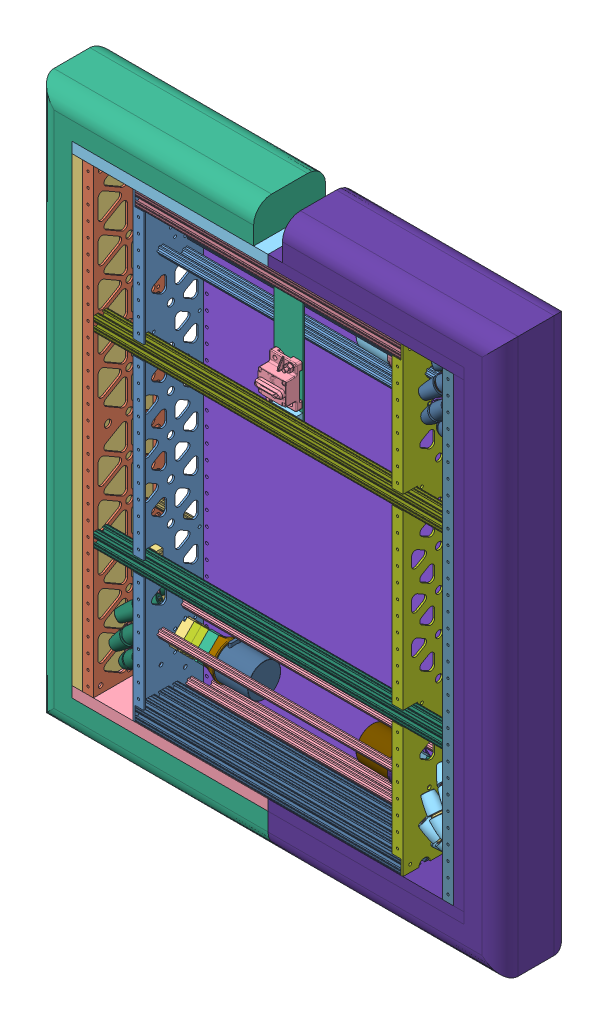
SolidWorks assembly Copy of Fame 2020, configuration Default. Lengths in mm.
Overall size (819.15 977.9 171.99).
407 component instances, 94 part files, 0 mates.
Components (placement in the parent):
- Inner plate v12(Mirror)^Copy of Fame 2020-1: Inner plate v12(Mirror)^Copy of Fame 2020 [Default] at (-212.725 0 58.7875) x (0 1 0) z (0 0 -1) size (812.8 19.05 127) (virtual)
  - Inner plate v12(Mirror)-0^Inner plate v12(Mirror)_Copy of Fame 2020-1: Inner plate v12(Mirror)-0^Inner plate v12(Mirror)_Copy of Fame 2020 [Default] at origin size (812.8 19.05 127) (virtual)
- Outer plate v11(Mirror)^Copy of Fame 2020-1: Outer plate v11(Mirror)^Copy of Fame 2020 [Default] at (-333.375 0 58.7875) x (0 -1 0) z (0 0 -1) size (812.8 19.05 127) (virtual)
  - Outer plate v11(Mirror)-1^Outer plate v11(Mirror)_Copy of Fame 2020-1: Outer plate v11(Mirror)-1^Outer plate v11(Mirror)_Copy of Fame 2020 [Default] at origin size (812.8 19.05 127) (virtual)
- Bumper Assembly v4(Mirror)^Copy of Fame 2020-1: Bumper Assembly v4(Mirror)^Copy of Fame 2020 [Default] at (-327.025 0.0665 58.7875) x (-1 0 0) z (0 0 -1) size (409.58 977.9 127) (virtual)
  - Bumper Assembly v4(Mirror)-2^Bumper Assembly v4(Mirror)_Copy of Fame 2020-1: Bumper Assembly v4(Mirror)-2^Bumper Assembly v4(Mirror)_Copy of Fame 2020 [Default] at origin size (19.05 812.8 127) (virtual)
  - Bumper Assembly v4(Mirror)-3^Bumper Assembly v4(Mirror)_Copy of Fame 2020-1: Bumper Assembly v4(Mirror)-3^Bumper Assembly v4(Mirror)_Copy of Fame 2020 [Default] at origin size (346.08 19.05 127) (virtual)
  - Bumper Assembly v4(Mirror)-4^Bumper Assembly v4(Mirror)_Copy of Fame 2020-1: Bumper Assembly v4(Mirror)-4^Bumper Assembly v4(Mirror)_Copy of Fame 2020 [Default] at origin size (346.08 19.05 127) (virtual)
  - Bumper Assembly v4(Mirror)-5^Bumper Assembly v4(Mirror)_Copy of Fame 2020-1: Bumper Assembly v4(Mirror)-5^Bumper Assembly v4(Mirror)_Copy of Fame 2020 [Default] at origin size (409.58 977.9 127) (virtual)
- NEO Gearbox 2-stage Custom^Copy of Fame 2020-1: NEO Gearbox 2-stage Custom^Copy of Fame 2020 [Default] at (0 0 425) size (164.9 90.53 90.53) (virtual)
  - VersaPlanetary_4_1_Gear_Kit_217-2818^NEO Gearbox 2-stage Custom_Copy of Fame 2020-1: VersaPlanetary_4_1_Gear_Kit_217-2818^NEO Gearbox 2-stage Custom_Copy of Fame 2020 [Default] at (-15.25 22.225 0) x (0 -0.707107 0.707107) z (-1 0 0) size (35.49 35.49 17.4) (virtual)
    - 217-2725-001 Rev1_24t Sun^VersaPlanetary_4_1_Gear_Kit_217-2818_NEO Gearbox 2-stage Custom_Copy of Fame 2020-1: 217-2725-001 Rev1_24t Sun^VersaPlanetary_4_1_Gear_Kit_217-2818_NEO Gearbox 2-stage Custom_Copy of Fame 2020 [Default] at (-36.69 -517.1337 -209.675) x (0.707107 0.707107 0) z (0 0 1) size (14.4 14.45 12.7) (virtual)
    - 217-2725-002 Rev1_24t Planet^VersaPlanetary_4_1_Gear_Kit_217-2818_NEO Gearbox 2-stage Custom_Copy of Fame 2020-1: 217-2725-002 Rev1_24t Planet^VersaPlanetary_4_1_Gear_Kit_217-2818_NEO Gearbox 2-stage Custom_Copy of Fame 2020 [Default] at (-45.2382 -525.6819 -212.025) x (-0.793353 0.608761 0) z (0 0 -1) size (13.12 13.1 8) (virtual)
    - 217-2724-002 Rev1^VersaPlanetary_4_1_Gear_Kit_217-2818_NEO Gearbox 2-stage Custom_Copy of Fame 2020-1: 217-2724-002 Rev1^VersaPlanetary_4_1_Gear_Kit_217-2818_NEO Gearbox 2-stage Custom_Copy of Fame 2020 [Default] at (-36.69 -517.1337 -218.375) x (1 0 0) z (0 0 -1) size (34.7 34.7 4.7) (virtual)
    - 217-2625-010 Rev1^VersaPlanetary_4_1_Gear_Kit_217-2818_NEO Gearbox 2-stage Custom_Copy of Fame 2020-1: 217-2625-010 Rev1^VersaPlanetary_4_1_Gear_Kit_217-2818_NEO Gearbox 2-stage Custom_Copy of Fame 2020 [Default] at (-45.2382 -525.6819 -214.725) x (0.854322 0.519745 0) z (0 0 1) size (4 4 12) (virtual)
    - 217-2725-002 Rev1_24t Planet^VersaPlanetary_4_1_Gear_Kit_217-2818_NEO Gearbox 2-stage Custom_Copy of Fame 2020-2: 217-2725-002 Rev1_24t Planet^VersaPlanetary_4_1_Gear_Kit_217-2818_NEO Gearbox 2-stage Custom_Copy of Fame 2020 [Default] at (-28.1418 -525.6819 -212.025) x (-0.608761 -0.793353 0) z (0 0 -1) size (13.12 13.1 8) (virtual)
    - 217-2725-002 Rev1_24t Planet^VersaPlanetary_4_1_Gear_Kit_217-2818_NEO Gearbox 2-stage Custom_Copy of Fame 2020-3: 217-2725-002 Rev1_24t Planet^VersaPlanetary_4_1_Gear_Kit_217-2818_NEO Gearbox 2-stage Custom_Copy of Fame 2020 [Default] at (-28.1418 -508.5855 -212.025) x (0.793353 -0.608761 0) z (0 0 -1) size (13.12 13.1 8) (virtual)
    - 217-2725-002 Rev1_24t Planet^VersaPlanetary_4_1_Gear_Kit_217-2818_NEO Gearbox 2-stage Custom_Copy of Fame 2020-4: 217-2725-002 Rev1_24t Planet^VersaPlanetary_4_1_Gear_Kit_217-2818_NEO Gearbox 2-stage Custom_Copy of Fame 2020 [Default] at (-45.2382 -508.5855 -212.025) x (0.608761 0.793353 0) z (0 0 -1) size (13.12 13.1 8) (virtual)
    - 217-2625-010 Rev1^VersaPlanetary_4_1_Gear_Kit_217-2818_NEO Gearbox 2-stage Custom_Copy of Fame 2020-2: 217-2625-010 Rev1^VersaPlanetary_4_1_Gear_Kit_217-2818_NEO Gearbox 2-stage Custom_Copy of Fame 2020 [Default] at (-28.1418 -525.6819 -214.725) x (-0.519745 0.854322 0) z (0 0 1) size (4 4 12) (virtual)
    - 217-2625-010 Rev1^VersaPlanetary_4_1_Gear_Kit_217-2818_NEO Gearbox 2-stage Custom_Copy of Fame 2020-3: 217-2625-010 Rev1^VersaPlanetary_4_1_Gear_Kit_217-2818_NEO Gearbox 2-stage Custom_Copy of Fame 2020 [Default] at (-28.1418 -508.5855 -214.725) x (-0.854322 -0.519745 0) z (0 0 1) size (4 4 12) (virtual)
    - 217-2625-010 Rev1^VersaPlanetary_4_1_Gear_Kit_217-2818_NEO Gearbox 2-stage Custom_Copy of Fame 2020-4: 217-2625-010 Rev1^VersaPlanetary_4_1_Gear_Kit_217-2818_NEO Gearbox 2-stage Custom_Copy of Fame 2020 [Default] at (-45.2382 -508.5855 -214.725) x (0.519745 -0.854322 0) z (0 0 1) size (4 4 12) (virtual)
  - 217-2625-026 Rev1^NEO Gearbox 2-stage Custom_Copy of Fame 2020-1: 217-2625-026 Rev1^NEO Gearbox 2-stage Custom_Copy of Fame 2020 [Default] at (211.875 -317.5 -391.6125) x (0 -0.707107 0.707107) z (-1 0 0) size (44.45 42 18.12) (virtual)
  - 217-2742-001 Rev4^NEO Gearbox 2-stage Custom_Copy of Fame 2020-1: 217-2742-001 Rev4^NEO Gearbox 2-stage Custom_Copy of Fame 2020 [Default] at (218.5752 -317.5 -391.6125) x (1 0 0) z (0 0.63857 0.769564) size (7 28 28) (virtual)
  - 217-2742-001 Rev4^NEO Gearbox 2-stage Custom_Copy of Fame 2020-2: 217-2742-001 Rev4^NEO Gearbox 2-stage Custom_Copy of Fame 2020 [Default] at (226.5752 -317.5 -391.6125) x (1 0 0) z (0 0.707107 0.707107) size (7 28 28) (virtual)
  - 217-2625-017 Rev1_9714K61^NEO Gearbox 2-stage Custom_Copy of Fame 2020-1: 217-2625-017 Rev1_9714K61^NEO Gearbox 2-stage Custom_Copy of Fame 2020 [Default] at (225.795 -317.6887 -391.9075) x (0 0.983393 0.181491) z (0 -0.181491 0.983393) size (28.51 4.98 27.43) (virtual)
  - 217-2625-025 Rev1^NEO Gearbox 2-stage Custom_Copy of Fame 2020-1: 217-2625-025 Rev1^NEO Gearbox 2-stage Custom_Copy of Fame 2020 [Default] at (182.475 -317.5 -391.6125) x (0 -0.707107 0.707107) z (-1 0 0) size (44.45 42 18) (virtual)
  - 217-2816-001 Rev1^NEO Gearbox 2-stage Custom_Copy of Fame 2020-1: 217-2816-001 Rev1^NEO Gearbox 2-stage Custom_Copy of Fame 2020 [Default] at (212.025 -317.5 -391.6125) x (0 -0.707107 0.707107) z (1 0 0) size (42 42 14.5) (virtual)
  - 217-2816-001 Rev1^NEO Gearbox 2-stage Custom_Copy of Fame 2020-2: 217-2816-001 Rev1^NEO Gearbox 2-stage Custom_Copy of Fame 2020 [Default] at (199.325 -317.5 -391.6125) x (0 -0.707107 0.707107) z (1 0 0) size (42 42 14.5) (virtual)
  - 217-4649-001 Rev1^NEO Gearbox 2-stage Custom_Copy of Fame 2020-1: 217-4649-001 Rev1^NEO Gearbox 2-stage Custom_Copy of Fame 2020 [Default] at (185.629 -317.5 -391.6125) x (0 -0.707107 0.707107) z (1 0 0) size (18 18 13) (virtual)
  - VersaPlanetary_CIM_Adapter_217-4018^NEO Gearbox 2-stage Custom_Copy of Fame 2020-1: VersaPlanetary_CIM_Adapter_217-4018^NEO Gearbox 2-stage Custom_Copy of Fame 2020 [Default] at (165.15 -317.5 -391.6125) x (0 -0.707107 0.707107) z (0 0.707107 0.707107) size (64.01 21.55 64.01) (virtual)
  - NEO Motor REV-21-1650^NEO Gearbox 2-stage Custom_Copy of Fame 2020-1: NEO Motor REV-21-1650^NEO Gearbox 2-stage Custom_Copy of Fame 2020 [Default] at (153.625 -317.5 -391.6125) x (0 -0.707107 -0.707107) z (1 0 0) size (61.14 61.02 93.25) (virtual)
  - 3_1 Output Shaft Custom^NEO Gearbox 2-stage Custom_Copy of Fame 2020-1: 3_1 Output Shaft Custom^NEO Gearbox 2-stage Custom_Copy of Fame 2020 [Default] at (211.3752 -317.5 -391.6125) x (1 0 0) z (0 0.707107 0.707107) size (48.9 34.7 34.7) (virtual)
- Left Wheel Assembly^Copy of Fame 2020-1: Left Wheel Assembly^Copy of Fame 2020 [Default] at (500 0 0) size (65.82 166.11 165.01) (virtual)
  - 6_Mecanum_Wheel_Left_217-2799^Left Wheel Assembly_Copy of Fame 2020-1: 6_Mecanum_Wheel_Left_217-2799^Left Wheel Assembly_Copy of Fame 2020 [Default] x (0 0 1) z (-1 0 0) size (165.01 166.11 65.82) (virtual)
    - 217-2799-001 Rev1^6_Mecanum_Wheel_Left_217-2799_Left Wheel Assembly_Copy of Fame 2020-1: 217-2799-001 Rev1^6_Mecanum_Wheel_Left_217-2799_Left Wheel Assembly_Copy of Fame 2020 [Default] at (33.3875 -317.5 234.0098) x (0.707107 0.707107 0) z (0 0 1) size (95.78 100.46 28.55) (virtual)
    - 217-2799-001 Rev1^6_Mecanum_Wheel_Left_217-2799_Left Wheel Assembly_Copy of Fame 2020-2: 217-2799-001 Rev1^6_Mecanum_Wheel_Left_217-2799_Left Wheel Assembly_Copy of Fame 2020 [Default] at (33.3875 -317.5 221.3098) x (-0.987688 -0.156434 0) z (0 0 -1) size (95.78 100.46 28.55) (virtual)
    - 217-2799-002 Rev1^6_Mecanum_Wheel_Left_217-2799_Left Wheel Assembly_Copy of Fame 2020-1: 217-2799-002 Rev1^6_Mecanum_Wheel_Left_217-2799_Left Wheel Assembly_Copy of Fame 2020 [Default] at (4.057 -346.8305 227.6598) x (-0.707107 0.707107 0) z (-0.707107 -0.707107 0) size (26.84 25.39 30.1) (virtual)
    - 217-2586-003 Rev2^6_Mecanum_Wheel_Left_217-2799_Left Wheel Assembly_Copy of Fame 2020-1: 217-2586-003 Rev2^6_Mecanum_Wheel_Left_217-2799_Left Wheel Assembly_Copy of Fame 2020 [Default] at (-13.4676 -358.6894 223.6536) x (0.41944 0.854155 0.30739) z (-0.757674 0.142894 0.636798) size (19.46 28.57 19.46) (virtual)
    - 217-2586-003 Rev2^6_Mecanum_Wheel_Left_217-2799_Left Wheel Assembly_Copy of Fame 2020-2: 217-2586-003 Rev2^6_Mecanum_Wheel_Left_217-2799_Left Wheel Assembly_Copy of Fame 2020 [Default] at (-7.8019 -364.3551 231.666) x (0.847342 0.451134 -0.280161) z (0.17892 -0.739241 -0.649238) size (19.46 28.57 19.46) (virtual)
    - 217-2586-004 Rev1^6_Mecanum_Wheel_Left_217-2799_Left Wheel Assembly_Copy of Fame 2020-1: 217-2586-004 Rev1^6_Mecanum_Wheel_Left_217-2799_Left Wheel Assembly_Copy of Fame 2020 [Default] at (-10.3479 -361.809 228.0654) x (-0.690521 -0.722949 -0.02293) z (0.522667 -0.476807 -0.706735) size (25.9 28.58 25.9) (virtual)
    - 217-2586-004 Rev1^6_Mecanum_Wheel_Left_217-2799_Left Wheel Assembly_Copy of Fame 2020-2: 217-2586-004 Rev1^6_Mecanum_Wheel_Left_217-2799_Left Wheel Assembly_Copy of Fame 2020 [Default] at (-10.9209 -361.2361 227.2551) x (0.01458 -0.811521 -0.584142) z (-0.865903 -0.302381 0.39847) size (25.9 28.58 25.9) (virtual)
    - 217-2586-007 Rev1^6_Mecanum_Wheel_Left_217-2799_Left Wheel Assembly_Copy of Fame 2020-1: 217-2586-007 Rev1^6_Mecanum_Wheel_Left_217-2799_Left Wheel Assembly_Copy of Fame 2020 [Default] at (-10.6347 -361.5222 227.6598) x (0.5 -0.5 0.707107) z (-0.709055 -0.705148 0.002763) size (61.72 5 5) (virtual)
    - 217-2586-008 Rev1^6_Mecanum_Wheel_Left_217-2799_Left Wheel Assembly_Copy of Fame 2020-1: 217-2586-008 Rev1^6_Mecanum_Wheel_Left_217-2799_Left Wheel Assembly_Copy of Fame 2020 [Default] at (53.3583 -330.4692 227.5328) x (0.544639 0.838671 0) z (0 0 -1) size (7.33 6.35 31.75) (virtual)
    - NUT-832-NYLOCK^6_Mecanum_Wheel_Left_217-2799_Left Wheel Assembly_Copy of Fame 2020-1: NUT-832-NYLOCK^6_Mecanum_Wheel_Left_217-2799_Left Wheel Assembly_Copy of Fame 2020 [Default] at (6.1639 -290.2764 241.3161) x (0.258819 -0.965926 0) z (-0.965926 -0.258819 0) size (9.37 5.86 8.12) (virtual)
    - SCREW-832-1250^6_Mecanum_Wheel_Left_217-2799_Left Wheel Assembly_Copy of Fame 2020-1: SCREW-832-1250^6_Mecanum_Wheel_Left_217-2799_Left Wheel Assembly_Copy of Fame 2020 [Default] at (6.1639 -290.2764 212.75) x (0 0 1) z (-0.394243 0.919006 0) size (33.96 7.92 7.92) (virtual)
    - 217-2586-007 Rev1^6_Mecanum_Wheel_Left_217-2799_Left Wheel Assembly_Copy of Fame 2020-2: 217-2586-007 Rev1^6_Mecanum_Wheel_Left_217-2799_Left Wheel Assembly_Copy of Fame 2020 [Default] at (-28.1029 -327.2391 227.6598) x (0.110616 -0.698401 0.707107) z (-0.988113 -0.153705 0.002763) size (61.72 5 5) (virtual)
    - 217-2586-007 Rev1^6_Mecanum_Wheel_Left_217-2799_Left Wheel Assembly_Copy of Fame 2020-3: 217-2586-007 Rev1^6_Mecanum_Wheel_Left_217-2799_Left Wheel Assembly_Copy of Fame 2020 [Default] at (-22.0838 -289.236 227.6598) x (-0.32102 -0.630037 0.707107) z (-0.889746 0.456448 0.002763) size (61.72 5 5) (virtual)
    - 217-2586-007 Rev1^6_Mecanum_Wheel_Left_217-2799_Left Wheel Assembly_Copy of Fame 2020-4: 217-2586-007 Rev1^6_Mecanum_Wheel_Left_217-2799_Left Wheel Assembly_Copy of Fame 2020 [Default] at (5.1235 -262.0287 227.6598) x (-0.630037 -0.32102 0.707107) z (-0.451526 0.892254 0.002763) size (61.72 5 5) (virtual)
    - 217-2586-007 Rev1^6_Mecanum_Wheel_Left_217-2799_Left Wheel Assembly_Copy of Fame 2020-5: 217-2586-007 Rev1^6_Mecanum_Wheel_Left_217-2799_Left Wheel Assembly_Copy of Fame 2020 [Default] at (43.1266 -256.0096 227.6598) x (-0.698401 0.110616 0.707107) z (0.159162 0.987249 0.002763) size (61.72 5 5) (virtual)
    - 217-2586-007 Rev1^6_Mecanum_Wheel_Left_217-2799_Left Wheel Assembly_Copy of Fame 2020-6: 217-2586-007 Rev1^6_Mecanum_Wheel_Left_217-2799_Left Wheel Assembly_Copy of Fame 2020 [Default] at (77.4097 -273.4778 227.6598) x (-0.5 0.5 0.707107) z (0.709055 0.705148 0.002763) size (61.72 5 5) (virtual)
    - 217-2586-007 Rev1^6_Mecanum_Wheel_Left_217-2799_Left Wheel Assembly_Copy of Fame 2020-7: 217-2586-007 Rev1^6_Mecanum_Wheel_Left_217-2799_Left Wheel Assembly_Copy of Fame 2020 [Default] at (94.8779 -307.7609 227.6598) x (-0.110616 0.698401 0.707107) z (0.988113 0.153705 0.002763) size (61.72 5 5) (virtual)
    - 217-2586-007 Rev1^6_Mecanum_Wheel_Left_217-2799_Left Wheel Assembly_Copy of Fame 2020-8: 217-2586-007 Rev1^6_Mecanum_Wheel_Left_217-2799_Left Wheel Assembly_Copy of Fame 2020 [Default] at (88.8588 -345.764 227.6598) x (0.32102 0.630037 0.707107) z (0.889746 -0.456448 0.002763) size (61.72 5 5) (virtual)
    - 217-2586-007 Rev1^6_Mecanum_Wheel_Left_217-2799_Left Wheel Assembly_Copy of Fame 2020-9: 217-2586-007 Rev1^6_Mecanum_Wheel_Left_217-2799_Left Wheel Assembly_Copy of Fame 2020 [Default] at (61.6515 -372.9713 227.6598) x (0.630037 0.32102 0.707107) z (0.451526 -0.892254 0.002763) size (61.72 5 5) (virtual)
    - 217-2586-007 Rev1^6_Mecanum_Wheel_Left_217-2799_Left Wheel Assembly_Copy of Fame 2020-10: 217-2586-007 Rev1^6_Mecanum_Wheel_Left_217-2799_Left Wheel Assembly_Copy of Fame 2020 [Default] at (23.6484 -378.9904 227.6598) x (0.698401 -0.110616 0.707107) z (-0.159162 -0.987249 0.002763) size (61.72 5 5) (virtual)
    - 217-2586-004 Rev1^6_Mecanum_Wheel_Left_217-2799_Left Wheel Assembly_Copy of Fame 2020-3: 217-2586-004 Rev1^6_Mecanum_Wheel_Left_217-2799_Left Wheel Assembly_Copy of Fame 2020 [Default] at (-28.1662 -326.8394 227.2551) x (-0.465204 -0.665104 -0.584142) z (-0.878265 0.264334 0.39847) size (25.9 28.58 25.9) (virtual)
    - 217-2586-004 Rev1^6_Mecanum_Wheel_Left_217-2799_Left Wheel Assembly_Copy of Fame 2020-4: 217-2586-004 Rev1^6_Mecanum_Wheel_Left_217-2799_Left Wheel Assembly_Copy of Fame 2020 [Default] at (-21.9 -288.8754 227.2551) x (-0.767297 -0.26464 -0.584142) z (-0.55516 0.730082 0.39847) size (25.9 28.58 25.9) (virtual)
    - 217-2586-004 Rev1^6_Mecanum_Wheel_Left_217-2799_Left Wheel Assembly_Copy of Fame 2020-5: 217-2586-004 Rev1^6_Mecanum_Wheel_Left_217-2799_Left Wheel Assembly_Copy of Fame 2020 [Default] at (5.484 -261.845 227.2551) x (-0.776308 0.236907 -0.584142) z (-0.020002 0.916963 0.39847) size (25.9 28.58 25.9) (virtual)
    - 217-2586-004 Rev1^6_Mecanum_Wheel_Left_217-2799_Left Wheel Assembly_Copy of Fame 2020-6: 217-2586-004 Rev1^6_Mecanum_Wheel_Left_217-2799_Left Wheel Assembly_Copy of Fame 2020 [Default] at (43.5263 -256.0729 227.2551) x (-0.488796 0.647964 -0.584142) z (0.522795 0.753596 0.39847) size (25.9 28.58 25.9) (virtual)
    - 217-2586-004 Rev1^6_Mecanum_Wheel_Left_217-2799_Left Wheel Assembly_Copy of Fame 2020-7: 217-2586-004 Rev1^6_Mecanum_Wheel_Left_217-2799_Left Wheel Assembly_Copy of Fame 2020 [Default] at (77.6959 -273.7639 227.2551) x (-0.01458 0.811521 -0.584142) z (0.865903 0.302381 0.39847) size (25.9 28.58 25.9) (virtual)
    - 217-2586-004 Rev1^6_Mecanum_Wheel_Left_217-2799_Left Wheel Assembly_Copy of Fame 2020-8: 217-2586-004 Rev1^6_Mecanum_Wheel_Left_217-2799_Left Wheel Assembly_Copy of Fame 2020 [Default] at (94.9412 -308.1606 227.2551) x (0.465204 0.665104 -0.584142) z (0.878265 -0.264334 0.39847) size (25.9 28.58 25.9) (virtual)
    - 217-2586-004 Rev1^6_Mecanum_Wheel_Left_217-2799_Left Wheel Assembly_Copy of Fame 2020-9: 217-2586-004 Rev1^6_Mecanum_Wheel_Left_217-2799_Left Wheel Assembly_Copy of Fame 2020 [Default] at (88.675 -346.1246 227.2551) x (0.767297 0.26464 -0.584142) z (0.55516 -0.730082 0.39847) size (25.9 28.58 25.9) (virtual)
    - 217-2586-004 Rev1^6_Mecanum_Wheel_Left_217-2799_Left Wheel Assembly_Copy of Fame 2020-10: 217-2586-004 Rev1^6_Mecanum_Wheel_Left_217-2799_Left Wheel Assembly_Copy of Fame 2020 [Default] at (61.291 -373.155 227.2551) x (0.776308 -0.236907 -0.584142) z (0.020002 -0.916963 0.39847) size (25.9 28.58 25.9) (virtual)
    - 217-2586-004 Rev1^6_Mecanum_Wheel_Left_217-2799_Left Wheel Assembly_Copy of Fame 2020-11: 217-2586-004 Rev1^6_Mecanum_Wheel_Left_217-2799_Left Wheel Assembly_Copy of Fame 2020 [Default] at (23.2487 -378.9271 227.2551) x (0.488796 -0.647964 -0.584142) z (-0.522795 -0.753596 0.39847) size (25.9 28.58 25.9) (virtual)
    - 217-2586-004 Rev1^6_Mecanum_Wheel_Left_217-2799_Left Wheel Assembly_Copy of Fame 2020-12: 217-2586-004 Rev1^6_Mecanum_Wheel_Left_217-2799_Left Wheel Assembly_Copy of Fame 2020 [Default] at (-28.0394 -327.6397 228.0654) x (-0.983582 -0.179 -0.02293) z (0.142587 -0.692961 -0.706735) size (25.9 28.58 25.9) (virtual)
    - 217-2586-004 Rev1^6_Mecanum_Wheel_Left_217-2799_Left Wheel Assembly_Copy of Fame 2020-13: 217-2586-004 Rev1^6_Mecanum_Wheel_Left_217-2799_Left Wheel Assembly_Copy of Fame 2020 [Default] at (-22.2679 -289.5974 228.0654) x (-0.900948 0.433321 -0.02293) z (-0.291957 -0.644427 -0.706735) size (25.9 28.58 25.9) (virtual)
    - 217-2586-004 Rev1^6_Mecanum_Wheel_Left_217-2799_Left Wheel Assembly_Copy of Fame 2020-14: 217-2586-004 Rev1^6_Mecanum_Wheel_Left_217-2799_Left Wheel Assembly_Copy of Fame 2020 [Default] at (4.7621 -262.2129 228.0654) x (-0.474183 0.880128 -0.02293) z (-0.614983 -0.349745 -0.706735) size (25.9 28.58 25.9) (virtual)
    - 217-2586-004 Rev1^6_Mecanum_Wheel_Left_217-2799_Left Wheel Assembly_Copy of Fame 2020-15: 217-2586-004 Rev1^6_Mecanum_Wheel_Left_217-2799_Left Wheel Assembly_Copy of Fame 2020 [Default] at (42.726 -255.9462 228.0654) x (0.133704 0.990756 -0.02293) z (-0.703107 0.078529 -0.706735) size (25.9 28.58 25.9) (virtual)
    - 217-2586-004 Rev1^6_Mecanum_Wheel_Left_217-2799_Left Wheel Assembly_Copy of Fame 2020-16: 217-2586-004 Rev1^6_Mecanum_Wheel_Left_217-2799_Left Wheel Assembly_Copy of Fame 2020 [Default] at (77.1229 -273.191 228.0654) x (0.690521 0.722949 -0.02293) z (-0.522667 0.476807 -0.706735) size (25.9 28.58 25.9) (virtual)
    - 217-2586-004 Rev1^6_Mecanum_Wheel_Left_217-2799_Left Wheel Assembly_Copy of Fame 2020-17: 217-2586-004 Rev1^6_Mecanum_Wheel_Left_217-2799_Left Wheel Assembly_Copy of Fame 2020 [Default] at (94.8144 -307.3603 228.0654) x (0.983582 0.179 -0.02293) z (-0.142587 0.692961 -0.706735) size (25.9 28.58 25.9) (virtual)
    - 217-2586-004 Rev1^6_Mecanum_Wheel_Left_217-2799_Left Wheel Assembly_Copy of Fame 2020-18: 217-2586-004 Rev1^6_Mecanum_Wheel_Left_217-2799_Left Wheel Assembly_Copy of Fame 2020 [Default] at (89.0429 -345.4026 228.0654) x (0.900948 -0.433321 -0.02293) z (0.291957 0.644427 -0.706735) size (25.9 28.58 25.9) (virtual)
    - 217-2586-004 Rev1^6_Mecanum_Wheel_Left_217-2799_Left Wheel Assembly_Copy of Fame 2020-19: 217-2586-004 Rev1^6_Mecanum_Wheel_Left_217-2799_Left Wheel Assembly_Copy of Fame 2020 [Default] at (62.0129 -372.7871 228.0654) x (0.474183 -0.880128 -0.02293) z (0.614983 0.349745 -0.706735) size (25.9 28.58 25.9) (virtual)
    - 217-2586-004 Rev1^6_Mecanum_Wheel_Left_217-2799_Left Wheel Assembly_Copy of Fame 2020-20: 217-2586-004 Rev1^6_Mecanum_Wheel_Left_217-2799_Left Wheel Assembly_Copy of Fame 2020 [Default] at (24.049 -379.0538 228.0654) x (-0.133704 -0.990756 -0.02293) z (0.703107 -0.078529 -0.706735) size (25.9 28.58 25.9) (virtual)
    - 217-2586-003 Rev2^6_Mecanum_Wheel_Left_217-2799_Left Wheel Assembly_Copy of Fame 2020-3: 217-2586-003 Rev2^6_Mecanum_Wheel_Left_217-2799_Left Wheel Assembly_Copy of Fame 2020 [Default] at (-27.4761 -331.196 231.666) x (0.950684 -0.13308 -0.280161) z (-0.289766 -0.703225 -0.649238) size (19.46 28.57 19.46) (virtual)
    - 217-2586-003 Rev2^6_Mecanum_Wheel_Left_217-2799_Left Wheel Assembly_Copy of Fame 2020-4: 217-2586-003 Rev2^6_Mecanum_Wheel_Left_217-2799_Left Wheel Assembly_Copy of Fame 2020 [Default] at (-23.9025 -292.8056 231.666) x (0.690897 -0.666462 -0.280161) z (-0.647771 -0.398601 -0.649238) size (19.46 28.57 19.46) (virtual)
    - 217-2586-003 Rev2^6_Mecanum_Wheel_Left_217-2799_Left Wheel Assembly_Copy of Fame 2020-5: 217-2586-003 Rev2^6_Mecanum_Wheel_Left_217-2799_Left Wheel Assembly_Copy of Fame 2020 [Default] at (1.5539 -263.8475 231.666) x (0.167211 -0.945278 -0.280161) z (-0.75835 0.058276 -0.649238) size (19.46 28.57 19.46) (virtual)
    - 217-2586-003 Rev2^6_Mecanum_Wheel_Left_217-2799_Left Wheel Assembly_Copy of Fame 2020-6: 217-2586-003 Rev2^6_Mecanum_Wheel_Left_217-2799_Left Wheel Assembly_Copy of Fame 2020 [Default] at (39.1697 -255.3829 231.666) x (-0.420344 -0.86303 -0.280161) z (-0.579264 0.492893 -0.649238) size (19.46 28.57 19.46) (virtual)
    - 217-2586-003 Rev2^6_Mecanum_Wheel_Left_217-2799_Left Wheel Assembly_Copy of Fame 2020-7: 217-2586-003 Rev2^6_Mecanum_Wheel_Left_217-2799_Left Wheel Assembly_Copy of Fame 2020 [Default] at (74.5769 -270.6449 231.666) x (-0.847342 -0.451134 -0.280161) z (-0.17892 0.739241 -0.649238) size (19.46 28.57 19.46) (virtual)
    - 217-2586-003 Rev2^6_Mecanum_Wheel_Left_217-2799_Left Wheel Assembly_Copy of Fame 2020-8: 217-2586-003 Rev2^6_Mecanum_Wheel_Left_217-2799_Left Wheel Assembly_Copy of Fame 2020 [Default] at (94.2511 -303.804 231.666) x (-0.950684 0.13308 -0.280161) z (0.289766 0.703225 -0.649238) size (19.46 28.57 19.46) (virtual)
    - 217-2586-003 Rev2^6_Mecanum_Wheel_Left_217-2799_Left Wheel Assembly_Copy of Fame 2020-9: 217-2586-003 Rev2^6_Mecanum_Wheel_Left_217-2799_Left Wheel Assembly_Copy of Fame 2020 [Default] at (90.6775 -342.1944 231.666) x (-0.690897 0.666462 -0.280161) z (0.647771 0.398601 -0.649238) size (19.46 28.57 19.46) (virtual)
    - 217-2586-003 Rev2^6_Mecanum_Wheel_Left_217-2799_Left Wheel Assembly_Copy of Fame 2020-10: 217-2586-003 Rev2^6_Mecanum_Wheel_Left_217-2799_Left Wheel Assembly_Copy of Fame 2020 [Default] at (65.2211 -371.1525 231.666) x (-0.167211 0.945278 -0.280161) z (0.75835 -0.058276 -0.649238) size (19.46 28.57 19.46) (virtual)
    - 217-2586-003 Rev2^6_Mecanum_Wheel_Left_217-2799_Left Wheel Assembly_Copy of Fame 2020-11: 217-2586-003 Rev2^6_Mecanum_Wheel_Left_217-2799_Left Wheel Assembly_Copy of Fame 2020 [Default] at (27.6053 -379.6171 231.666) x (0.420344 0.86303 -0.280161) z (0.579264 -0.492893 -0.649238) size (19.46 28.57 19.46) (virtual)
    - 217-2586-003 Rev2^6_Mecanum_Wheel_Left_217-2799_Left Wheel Assembly_Copy of Fame 2020-12: 217-2586-003 Rev2^6_Mecanum_Wheel_Left_217-2799_Left Wheel Assembly_Copy of Fame 2020 [Default] at (-28.7296 -323.2822 223.6536) x (0.841394 0.444485 0.30739) z (-0.52898 0.560953 0.636798) size (19.46 28.57 19.46) (virtual)
    - 217-2586-003 Rev2^6_Mecanum_Wheel_Left_217-2799_Left Wheel Assembly_Copy of Fame 2020-13: 217-2586-003 Rev2^6_Mecanum_Wheel_Left_217-2799_Left Wheel Assembly_Copy of Fame 2020 [Default] at (-20.265 -285.6664 223.6536) x (0.941964 -0.134963 0.30739) z (-0.098234 0.764747 0.636798) size (19.46 28.57 19.46) (virtual)
    - 217-2586-003 Rev2^6_Mecanum_Wheel_Left_217-2799_Left Wheel Assembly_Copy of Fame 2020-14: 217-2586-003 Rev2^6_Mecanum_Wheel_Left_217-2799_Left Wheel Assembly_Copy of Fame 2020 [Default] at (8.6931 -260.21 223.6536) x (0.682736 -0.66286 0.30739) z (0.370035 0.676434 0.636798) size (19.46 28.57 19.46) (virtual)
    - 217-2586-003 Rev2^6_Mecanum_Wheel_Left_217-2799_Left Wheel Assembly_Copy of Fame 2020-15: 217-2586-003 Rev2^6_Mecanum_Wheel_Left_217-2799_Left Wheel Assembly_Copy of Fame 2020 [Default] at (47.0835 -256.6364 223.6536) x (0.162726 -0.937567 0.30739) z (0.696962 0.329746 0.636798) size (19.46 28.57 19.46) (virtual)
    - 217-2586-003 Rev2^6_Mecanum_Wheel_Left_217-2799_Left Wheel Assembly_Copy of Fame 2020-16: 217-2586-003 Rev2^6_Mecanum_Wheel_Left_217-2799_Left Wheel Assembly_Copy of Fame 2020 [Default] at (80.2426 -276.3106 223.6536) x (-0.41944 -0.854155 0.30739) z (0.757674 -0.142894 0.636798) size (19.46 28.57 19.46) (virtual)
    - 217-2586-003 Rev2^6_Mecanum_Wheel_Left_217-2799_Left Wheel Assembly_Copy of Fame 2020-17: 217-2586-003 Rev2^6_Mecanum_Wheel_Left_217-2799_Left Wheel Assembly_Copy of Fame 2020 [Default] at (95.5046 -311.7178 223.6536) x (-0.841394 -0.444485 0.30739) z (0.52898 -0.560953 0.636798) size (19.46 28.57 19.46) (virtual)
    - 217-2586-003 Rev2^6_Mecanum_Wheel_Left_217-2799_Left Wheel Assembly_Copy of Fame 2020-18: 217-2586-003 Rev2^6_Mecanum_Wheel_Left_217-2799_Left Wheel Assembly_Copy of Fame 2020 [Default] at (87.04 -349.3336 223.6536) x (-0.941964 0.134963 0.30739) z (0.098234 -0.764747 0.636798) size (19.46 28.57 19.46) (virtual)
    - 217-2586-003 Rev2^6_Mecanum_Wheel_Left_217-2799_Left Wheel Assembly_Copy of Fame 2020-19: 217-2586-003 Rev2^6_Mecanum_Wheel_Left_217-2799_Left Wheel Assembly_Copy of Fame 2020 [Default] at (58.0819 -374.79 223.6536) x (-0.682736 0.66286 0.30739) z (-0.370035 -0.676434 0.636798) size (19.46 28.57 19.46) (virtual)
    - 217-2586-003 Rev2^6_Mecanum_Wheel_Left_217-2799_Left Wheel Assembly_Copy of Fame 2020-20: 217-2586-003 Rev2^6_Mecanum_Wheel_Left_217-2799_Left Wheel Assembly_Copy of Fame 2020 [Default] at (19.6915 -378.3636 223.6536) x (-0.162726 0.937567 0.30739) z (-0.696962 -0.329746 0.636798) size (19.46 28.57 19.46) (virtual)
    - 217-2799-002 Rev1^6_Mecanum_Wheel_Left_217-2799_Left Wheel Assembly_Copy of Fame 2020-2: 217-2799-002 Rev1^6_Mecanum_Wheel_Left_217-2799_Left Wheel Assembly_Copy of Fame 2020 [Default] at (-7.5815 -323.9888 227.6598) x (-0.156434 0.987688 0) z (-0.987688 -0.156434 0) size (26.84 25.39 30.1) (virtual)
    - 217-2799-002 Rev1^6_Mecanum_Wheel_Left_217-2799_Left Wheel Assembly_Copy of Fame 2020-3: 217-2799-002 Rev1^6_Mecanum_Wheel_Left_217-2799_Left Wheel Assembly_Copy of Fame 2020 [Default] at (-3.5711 -298.6686 227.6598) x (0.45399 0.891007 0) z (-0.891007 0.45399 0) size (26.84 25.39 30.1) (virtual)
    - 217-2799-002 Rev1^6_Mecanum_Wheel_Left_217-2799_Left Wheel Assembly_Copy of Fame 2020-4: 217-2799-002 Rev1^6_Mecanum_Wheel_Left_217-2799_Left Wheel Assembly_Copy of Fame 2020 [Default] at (14.5561 -280.5414 227.6598) x (0.891007 0.45399 0) z (-0.45399 0.891007 0) size (26.84 25.39 30.1) (virtual)
    - 217-2799-002 Rev1^6_Mecanum_Wheel_Left_217-2799_Left Wheel Assembly_Copy of Fame 2020-5: 217-2799-002 Rev1^6_Mecanum_Wheel_Left_217-2799_Left Wheel Assembly_Copy of Fame 2020 [Default] at (39.8763 -276.531 227.6598) x (0.987688 -0.156434 0) z (0.156434 0.987688 0) size (26.84 25.39 30.1) (virtual)
    - 217-2799-002 Rev1^6_Mecanum_Wheel_Left_217-2799_Left Wheel Assembly_Copy of Fame 2020-6: 217-2799-002 Rev1^6_Mecanum_Wheel_Left_217-2799_Left Wheel Assembly_Copy of Fame 2020 [Default] at (62.718 -288.1695 227.6598) x (0.707107 -0.707107 0) z (0.707107 0.707107 0) size (26.84 25.39 30.1) (virtual)
    - 217-2799-002 Rev1^6_Mecanum_Wheel_Left_217-2799_Left Wheel Assembly_Copy of Fame 2020-7: 217-2799-002 Rev1^6_Mecanum_Wheel_Left_217-2799_Left Wheel Assembly_Copy of Fame 2020 [Default] at (74.3565 -311.0112 227.6598) x (0.156434 -0.987688 0) z (0.987688 0.156434 0) size (26.84 25.39 30.1) (virtual)
    - 217-2799-002 Rev1^6_Mecanum_Wheel_Left_217-2799_Left Wheel Assembly_Copy of Fame 2020-8: 217-2799-002 Rev1^6_Mecanum_Wheel_Left_217-2799_Left Wheel Assembly_Copy of Fame 2020 [Default] at (70.3461 -336.3314 227.6598) x (-0.45399 -0.891007 0) z (0.891007 -0.45399 0) size (26.84 25.39 30.1) (virtual)
    - 217-2799-002 Rev1^6_Mecanum_Wheel_Left_217-2799_Left Wheel Assembly_Copy of Fame 2020-9: 217-2799-002 Rev1^6_Mecanum_Wheel_Left_217-2799_Left Wheel Assembly_Copy of Fame 2020 [Default] at (52.2189 -354.4586 227.6598) x (-0.891007 -0.45399 0) z (0.45399 -0.891007 0) size (26.84 25.39 30.1) (virtual)
    - 217-2799-002 Rev1^6_Mecanum_Wheel_Left_217-2799_Left Wheel Assembly_Copy of Fame 2020-10: 217-2799-002 Rev1^6_Mecanum_Wheel_Left_217-2799_Left Wheel Assembly_Copy of Fame 2020 [Default] at (26.8987 -358.469 227.6598) x (-0.987688 0.156434 0) z (-0.156434 -0.987688 0) size (26.84 25.39 30.1) (virtual)
    - 217-2586-008 Rev1^6_Mecanum_Wheel_Left_217-2799_Left Wheel Assembly_Copy of Fame 2020-2: 217-2586-008 Rev1^6_Mecanum_Wheel_Left_217-2799_Left Wheel Assembly_Copy of Fame 2020 [Default] at (32.1413 -341.2799 227.5328) x (0.99863 -0.052336 0) z (0 0 -1) size (7.33 6.35 31.75) (virtual)
    - 217-2586-008 Rev1^6_Mecanum_Wheel_Left_217-2799_Left Wheel Assembly_Copy of Fame 2020-3: 217-2586-008 Rev1^6_Mecanum_Wheel_Left_217-2799_Left Wheel Assembly_Copy of Fame 2020 [Default] at (12.1704 -328.3106 227.5328) x (0.45399 -0.891007 0) z (0 0 -1) size (7.33 6.35 31.75) (virtual)
    - 217-2586-008 Rev1^6_Mecanum_Wheel_Left_217-2799_Left Wheel Assembly_Copy of Fame 2020-4: 217-2586-008 Rev1^6_Mecanum_Wheel_Left_217-2799_Left Wheel Assembly_Copy of Fame 2020 [Default] at (13.4167 -304.5308 227.5328) x (-0.544639 -0.838671 0) z (0 0 -1) size (7.33 6.35 31.75) (virtual)
    - 217-2586-008 Rev1^6_Mecanum_Wheel_Left_217-2799_Left Wheel Assembly_Copy of Fame 2020-5: 217-2586-008 Rev1^6_Mecanum_Wheel_Left_217-2799_Left Wheel Assembly_Copy of Fame 2020 [Default] at (34.6337 -293.7201 227.5328) x (-0.99863 0.052336 0) z (0 0 -1) size (7.33 6.35 31.75) (virtual)
    - 217-2586-008 Rev1^6_Mecanum_Wheel_Left_217-2799_Left Wheel Assembly_Copy of Fame 2020-6: 217-2586-008 Rev1^6_Mecanum_Wheel_Left_217-2799_Left Wheel Assembly_Copy of Fame 2020 [Default] at (54.6046 -306.6894 227.5328) x (-0.45399 0.891007 0) z (0 0 -1) size (7.33 6.35 31.75) (virtual)
    - SCREW-832-1250^6_Mecanum_Wheel_Left_217-2799_Left Wheel Assembly_Copy of Fame 2020-2: SCREW-832-1250^6_Mecanum_Wheel_Left_217-2799_Left Wheel Assembly_Copy of Fame 2020 [Default] at (-0.9163 -334.9786 212.75) x (0 0 1) z (-0.995855 -0.090959 0) size (33.96 7.92 7.92) (virtual)
    - SCREW-832-1250^6_Mecanum_Wheel_Left_217-2799_Left Wheel Assembly_Copy of Fame 2020-3: SCREW-832-1250^6_Mecanum_Wheel_Left_217-2799_Left Wheel Assembly_Copy of Fame 2020 [Default] at (39.4102 -355.526 212.75) x (0 0 1) z (-0.221229 -0.975222 0) size (33.96 7.92 7.92) (virtual)
    - SCREW-832-1250^6_Mecanum_Wheel_Left_217-2799_Left Wheel Assembly_Copy of Fame 2020-4: SCREW-832-1250^6_Mecanum_Wheel_Left_217-2799_Left Wheel Assembly_Copy of Fame 2020 [Default] at (71.4135 -323.5227 212.75) x (0 0 1) z (0.859128 -0.511761 0) size (33.96 7.92 7.92) (virtual)
    - SCREW-832-1250^6_Mecanum_Wheel_Left_217-2799_Left Wheel Assembly_Copy of Fame 2020-5: SCREW-832-1250^6_Mecanum_Wheel_Left_217-2799_Left Wheel Assembly_Copy of Fame 2020 [Default] at (50.8661 -283.1962 212.75) x (0 0 1) z (0.752199 0.658936 0) size (33.96 7.92 7.92) (virtual)
    - NUT-832-NYLOCK^6_Mecanum_Wheel_Left_217-2799_Left Wheel Assembly_Copy of Fame 2020-2: NUT-832-NYLOCK^6_Mecanum_Wheel_Left_217-2799_Left Wheel Assembly_Copy of Fame 2020 [Default] at (-0.9163 -334.9786 241.3161) x (0.99863 -0.052336 0) z (-0.052336 -0.99863 0) size (9.37 5.86 8.12) (virtual)
    - NUT-832-NYLOCK^6_Mecanum_Wheel_Left_217-2799_Left Wheel Assembly_Copy of Fame 2020-3: NUT-832-NYLOCK^6_Mecanum_Wheel_Left_217-2799_Left Wheel Assembly_Copy of Fame 2020 [Default] at (39.4102 -355.526 241.3161) x (0.358368 0.93358 0) z (0.93358 -0.358368 0) size (9.37 5.86 8.12) (virtual)
    - NUT-832-NYLOCK^6_Mecanum_Wheel_Left_217-2799_Left Wheel Assembly_Copy of Fame 2020-4: NUT-832-NYLOCK^6_Mecanum_Wheel_Left_217-2799_Left Wheel Assembly_Copy of Fame 2020 [Default] at (71.4135 -323.5227 241.3161) x (-0.777146 0.62932 0) z (0.62932 0.777146 0) size (9.37 5.86 8.12) (virtual)
    - NUT-832-NYLOCK^6_Mecanum_Wheel_Left_217-2799_Left Wheel Assembly_Copy of Fame 2020-5: NUT-832-NYLOCK^6_Mecanum_Wheel_Left_217-2799_Left Wheel Assembly_Copy of Fame 2020 [Default] at (50.8661 -283.1962 241.3161) x (-0.838671 -0.544639 0) z (-0.544639 0.838671 0) size (9.37 5.86 8.12) (virtual)
    - 217-2586-005 Rev2^6_Mecanum_Wheel_Left_217-2799_Left Wheel Assembly_Copy of Fame 2020-1: 217-2586-005 Rev2^6_Mecanum_Wheel_Left_217-2799_Left Wheel Assembly_Copy of Fame 2020 [Default] at (-6.1597 -365.9972 233.9884) x (-0.5 0.5 -0.707107) z (0.146447 0.853553 0.5) size (8.5 8 8) (virtual)
    - 217-2586-005 Rev2^6_Mecanum_Wheel_Left_217-2799_Left Wheel Assembly_Copy of Fame 2020-2: 217-2586-005 Rev2^6_Mecanum_Wheel_Left_217-2799_Left Wheel Assembly_Copy of Fame 2020 [Default] at (-15.1097 -357.0472 221.3312) x (-0.5 0.5 -0.707107) z (0.146447 0.853553 0.5) size (8.5 8 8) (virtual)
    - 217-2586-005 Rev2^6_Mecanum_Wheel_Left_217-2799_Left Wheel Assembly_Copy of Fame 2020-3: 217-2586-005 Rev2^6_Mecanum_Wheel_Left_217-2799_Left Wheel Assembly_Copy of Fame 2020 [Default] at (-29.0929 -320.9884 221.3312) x (-0.110616 0.698401 -0.707107) z (0.620184 0.60446 0.5) size (8.5 8 8) (virtual)
    - 217-2586-005 Rev2^6_Mecanum_Wheel_Left_217-2799_Left Wheel Assembly_Copy of Fame 2020-4: 217-2586-005 Rev2^6_Mecanum_Wheel_Left_217-2799_Left Wheel Assembly_Copy of Fame 2020 [Default] at (-19.2106 -283.5972 221.3312) x (0.32102 0.630037 -0.707107) z (0.857032 0.124484 0.5) size (8.5 8 8) (virtual)
    - 217-2586-005 Rev2^6_Mecanum_Wheel_Left_217-2799_Left Wheel Assembly_Copy of Fame 2020-5: 217-2586-005 Rev2^6_Mecanum_Wheel_Left_217-2799_Left Wheel Assembly_Copy of Fame 2020 [Default] at (10.7623 -259.1556 221.3312) x (0.630037 0.32102 -0.707107) z (0.766523 -0.403042 0.5) size (8.5 8 8) (virtual)
    - 217-2586-005 Rev2^6_Mecanum_Wheel_Left_217-2799_Left Wheel Assembly_Copy of Fame 2020-6: 217-2586-005 Rev2^6_Mecanum_Wheel_Left_217-2799_Left Wheel Assembly_Copy of Fame 2020 [Default] at (49.3773 -256.9997 221.3312) x (0.698401 -0.110616 -0.707107) z (0.383228 -0.776618 0.5) size (8.5 8 8) (virtual)
    - 217-2586-005 Rev2^6_Mecanum_Wheel_Left_217-2799_Left Wheel Assembly_Copy of Fame 2020-7: 217-2586-005 Rev2^6_Mecanum_Wheel_Left_217-2799_Left Wheel Assembly_Copy of Fame 2020 [Default] at (81.8847 -277.9528 221.3312) x (0.5 -0.5 -0.707107) z (-0.146447 -0.853553 0.5) size (8.5 8 8) (virtual)
    - 217-2586-005 Rev2^6_Mecanum_Wheel_Left_217-2799_Left Wheel Assembly_Copy of Fame 2020-8: 217-2586-005 Rev2^6_Mecanum_Wheel_Left_217-2799_Left Wheel Assembly_Copy of Fame 2020 [Default] at (95.8679 -314.0116 221.3312) x (0.110616 -0.698401 -0.707107) z (-0.620184 -0.60446 0.5) size (8.5 8 8) (virtual)
    - 217-2586-005 Rev2^6_Mecanum_Wheel_Left_217-2799_Left Wheel Assembly_Copy of Fame 2020-9: 217-2586-005 Rev2^6_Mecanum_Wheel_Left_217-2799_Left Wheel Assembly_Copy of Fame 2020 [Default] at (85.9856 -351.4028 221.3312) x (-0.32102 -0.630037 -0.707107) z (-0.857032 -0.124484 0.5) size (8.5 8 8) (virtual)
    - 217-2586-005 Rev2^6_Mecanum_Wheel_Left_217-2799_Left Wheel Assembly_Copy of Fame 2020-10: 217-2586-005 Rev2^6_Mecanum_Wheel_Left_217-2799_Left Wheel Assembly_Copy of Fame 2020 [Default] at (56.0127 -375.8444 221.3312) x (-0.630037 -0.32102 -0.707107) z (-0.766523 0.403042 0.5) size (8.5 8 8) (virtual)
    - 217-2586-005 Rev2^6_Mecanum_Wheel_Left_217-2799_Left Wheel Assembly_Copy of Fame 2020-11: 217-2586-005 Rev2^6_Mecanum_Wheel_Left_217-2799_Left Wheel Assembly_Copy of Fame 2020 [Default] at (17.3977 -378.0003 221.3312) x (-0.698401 0.110616 -0.707107) z (-0.383228 0.776618 0.5) size (8.5 8 8) (virtual)
    - 217-2586-005 Rev2^6_Mecanum_Wheel_Left_217-2799_Left Wheel Assembly_Copy of Fame 2020-12: 217-2586-005 Rev2^6_Mecanum_Wheel_Left_217-2799_Left Wheel Assembly_Copy of Fame 2020 [Default] at (-27.1128 -333.4898 233.9884) x (-0.110616 0.698401 -0.707107) z (0.620184 0.60446 0.5) size (8.5 8 8) (virtual)
    - 217-2586-005 Rev2^6_Mecanum_Wheel_Left_217-2799_Left Wheel Assembly_Copy of Fame 2020-13: 217-2586-005 Rev2^6_Mecanum_Wheel_Left_217-2799_Left Wheel Assembly_Copy of Fame 2020 [Default] at (-24.9569 -294.8748 233.9884) x (0.32102 0.630037 -0.707107) z (0.857032 0.124484 0.5) size (8.5 8 8) (virtual)
    - 217-2586-005 Rev2^6_Mecanum_Wheel_Left_217-2799_Left Wheel Assembly_Copy of Fame 2020-14: 217-2586-005 Rev2^6_Mecanum_Wheel_Left_217-2799_Left Wheel Assembly_Copy of Fame 2020 [Default] at (-0.5153 -264.9019 233.9884) x (0.630037 0.32102 -0.707107) z (0.766523 -0.403042 0.5) size (8.5 8 8) (virtual)
    - 217-2586-005 Rev2^6_Mecanum_Wheel_Left_217-2799_Left Wheel Assembly_Copy of Fame 2020-15: 217-2586-005 Rev2^6_Mecanum_Wheel_Left_217-2799_Left Wheel Assembly_Copy of Fame 2020 [Default] at (36.8759 -255.0196 233.9884) x (0.698401 -0.110616 -0.707107) z (0.383228 -0.776618 0.5) size (8.5 8 8) (virtual)
    - 217-2586-005 Rev2^6_Mecanum_Wheel_Left_217-2799_Left Wheel Assembly_Copy of Fame 2020-16: 217-2586-005 Rev2^6_Mecanum_Wheel_Left_217-2799_Left Wheel Assembly_Copy of Fame 2020 [Default] at (72.9347 -269.0028 233.9884) x (0.5 -0.5 -0.707107) z (-0.146447 -0.853553 0.5) size (8.5 8 8) (virtual)
    - 217-2586-005 Rev2^6_Mecanum_Wheel_Left_217-2799_Left Wheel Assembly_Copy of Fame 2020-17: 217-2586-005 Rev2^6_Mecanum_Wheel_Left_217-2799_Left Wheel Assembly_Copy of Fame 2020 [Default] at (93.8878 -301.5102 233.9884) x (0.110616 -0.698401 -0.707107) z (-0.620184 -0.60446 0.5) size (8.5 8 8) (virtual)
    - 217-2586-005 Rev2^6_Mecanum_Wheel_Left_217-2799_Left Wheel Assembly_Copy of Fame 2020-18: 217-2586-005 Rev2^6_Mecanum_Wheel_Left_217-2799_Left Wheel Assembly_Copy of Fame 2020 [Default] at (91.7319 -340.1252 233.9884) x (-0.32102 -0.630037 -0.707107) z (-0.857032 -0.124484 0.5) size (8.5 8 8) (virtual)
    - 217-2586-005 Rev2^6_Mecanum_Wheel_Left_217-2799_Left Wheel Assembly_Copy of Fame 2020-19: 217-2586-005 Rev2^6_Mecanum_Wheel_Left_217-2799_Left Wheel Assembly_Copy of Fame 2020 [Default] at (67.2903 -370.0981 233.9884) x (-0.630037 -0.32102 -0.707107) z (-0.766523 0.403042 0.5) size (8.5 8 8) (virtual)
    - 217-2586-005 Rev2^6_Mecanum_Wheel_Left_217-2799_Left Wheel Assembly_Copy of Fame 2020-20: 217-2586-005 Rev2^6_Mecanum_Wheel_Left_217-2799_Left Wheel Assembly_Copy of Fame 2020 [Default] at (29.8991 -379.9804 233.9884) x (-0.698401 0.110616 -0.707107) z (-0.383228 0.776618 0.5) size (8.5 8 8) (virtual)
  - 1_2_Hex_Bore_Aluminum_VersaHub_217-2592^Left Wheel Assembly_Copy of Fame 2020-1: 1_2_Hex_Bore_Aluminum_VersaHub_217-2592^Left Wheel Assembly_Copy of Fame 2020 [Default] at (-239.7248 -317.5 33.3875) x (-1 0 0) z (0 0.707107 0.707107) size (12.7 55.88 55.88) (virtual)
- NEO Gearbox 2-stage Custom v5(Mirror) (2)^Copy of Fame 2020-1: NEO Gearbox 2-stage Custom v5(Mirror) (2)^Copy of Fame 2020 [Default] at (0 0 425) x (1 0 0) z (0 0 -1) size (164.9 90.53 90.53) (virtual)
  - VersaPlanetary_4_1_Gear_Kit_217-2818 v1(Mirror) (2)^NEO Gearbox 2-stage Custom v5(Mirror) (2)_Copy of Fame 2020-1: VersaPlanetary_4_1_Gear_Kit_217-2818 v1(Mirror) (2)^NEO Gearbox 2-stage Custom v5(Mirror) (2)_Copy of Fame 2020 [Default] at (-15.25 22.225 0) x (0 -0.707107 -0.707107) z (1 0 0) size (35.49 35.49 17.4) (virtual)
    - 217-2725-001 Rev1_24t Sun(Mirror) (2)^VersaPlanetary_4_1_Gear_Kit_217-2818 v1(Mirror) (2)_NEO Gearbox 2-stage Custom v5(Mirror) (2)_Copy of Fame 2020-1: 217-2725-001 Rev1_24t Sun(Mirror) (2)^VersaPlanetary_4_1_Gear_Kit_217-2818 v1(Mirror) (2)_NEO Gearbox 2-stage Custom v5(Mirror) (2)_Copy of Fame 2020 [Default] at (-36.69 -517.1337 209.675) x (0.707107 0.707107 0) z (0 0 1) size (14.4 14.45 12.7) (virtual)
    - 217-2725-002 Rev1_24t Planet(Mirror) (2)^VersaPlanetary_4_1_Gear_Kit_217-2818 v1(Mirror) (2)_NEO Gearbox 2-stage Custom v5(Mirror) (2)_Copy of Fame 2020-1: 217-2725-002 Rev1_24t Planet(Mirror) (2)^VersaPlanetary_4_1_Gear_Kit_217-2818 v1(Mirror) (2)_NEO Gearbox 2-stage Custom v5(Mirror) (2)_Copy of Fame 2020 [Default] at (-45.2382 -525.6819 212.025) x (-0.793353 0.608761 0) z (0 0 -1) size (13.12 13.1 8) (virtual)
    - 217-2725-002 Rev1_24t Planet(Mirror) (2)^VersaPlanetary_4_1_Gear_Kit_217-2818 v1(Mirror) (2)_NEO Gearbox 2-stage Custom v5(Mirror) (2)_Copy of Fame 2020-2: 217-2725-002 Rev1_24t Planet(Mirror) (2)^VersaPlanetary_4_1_Gear_Kit_217-2818 v1(Mirror) (2)_NEO Gearbox 2-stage Custom v5(Mirror) (2)_Copy of Fame 2020 [Default] at (-28.1418 -525.6819 212.025) x (-0.608761 -0.793353 0) z (0 0 -1) size (13.12 13.1 8) (virtual)
    - 217-2725-002 Rev1_24t Planet(Mirror) (2)^VersaPlanetary_4_1_Gear_Kit_217-2818 v1(Mirror) (2)_NEO Gearbox 2-stage Custom v5(Mirror) (2)_Copy of Fame 2020-3: 217-2725-002 Rev1_24t Planet(Mirror) (2)^VersaPlanetary_4_1_Gear_Kit_217-2818 v1(Mirror) (2)_NEO Gearbox 2-stage Custom v5(Mirror) (2)_Copy of Fame 2020 [Default] at (-28.1418 -508.5855 212.025) x (0.793353 -0.608761 0) z (0 0 -1) size (13.12 13.1 8) (virtual)
    - 217-2725-002 Rev1_24t Planet(Mirror) (2)^VersaPlanetary_4_1_Gear_Kit_217-2818 v1(Mirror) (2)_NEO Gearbox 2-stage Custom v5(Mirror) (2)_Copy of Fame 2020-4: 217-2725-002 Rev1_24t Planet(Mirror) (2)^VersaPlanetary_4_1_Gear_Kit_217-2818 v1(Mirror) (2)_NEO Gearbox 2-stage Custom v5(Mirror) (2)_Copy of Fame 2020 [Default] at (-45.2382 -508.5855 212.025) x (0.608761 0.793353 0) z (0 0 -1) size (13.12 13.1 8) (virtual)
    - 217-2724-002 Rev1(Mirror) (2)^VersaPlanetary_4_1_Gear_Kit_217-2818 v1(Mirror) (2)_NEO Gearbox 2-stage Custom v5(Mirror) (2)_Copy of Fame 2020-1: 217-2724-002 Rev1(Mirror) (2)^VersaPlanetary_4_1_Gear_Kit_217-2818 v1(Mirror) (2)_NEO Gearbox 2-stage Custom v5(Mirror) (2)_Copy of Fame 2020 [Default] at (-36.69 -517.1337 218.375) x (1 0 0) z (0 0 -1) size (34.7 34.7 4.7) (virtual)
    - 217-2625-010 Rev1(Mirror) (2)^VersaPlanetary_4_1_Gear_Kit_217-2818 v1(Mirror) (2)_NEO Gearbox 2-stage Custom v5(Mirror) (2)_Copy of Fame 2020-1: 217-2625-010 Rev1(Mirror) (2)^VersaPlanetary_4_1_Gear_Kit_217-2818 v1(Mirror) (2)_NEO Gearbox 2-stage Custom v5(Mirror) (2)_Copy of Fame 2020 [Default] at (-45.2382 -525.6819 214.725) x (0.854322 0.519745 0) z (0 0 1) size (4 4 12) (virtual)
    - 217-2625-010 Rev1(Mirror) (2)^VersaPlanetary_4_1_Gear_Kit_217-2818 v1(Mirror) (2)_NEO Gearbox 2-stage Custom v5(Mirror) (2)_Copy of Fame 2020-2: 217-2625-010 Rev1(Mirror) (2)^VersaPlanetary_4_1_Gear_Kit_217-2818 v1(Mirror) (2)_NEO Gearbox 2-stage Custom v5(Mirror) (2)_Copy of Fame 2020 [Default] at (-28.1418 -525.6819 214.725) x (-0.519745 0.854322 0) z (0 0 1) size (4 4 12) (virtual)
    - 217-2625-010 Rev1(Mirror) (2)^VersaPlanetary_4_1_Gear_Kit_217-2818 v1(Mirror) (2)_NEO Gearbox 2-stage Custom v5(Mirror) (2)_Copy of Fame 2020-3: 217-2625-010 Rev1(Mirror) (2)^VersaPlanetary_4_1_Gear_Kit_217-2818 v1(Mirror) (2)_NEO Gearbox 2-stage Custom v5(Mirror) (2)_Copy of Fame 2020 [Default] at (-28.1418 -508.5855 214.725) x (-0.854322 -0.519745 0) z (0 0 1) size (4 4 12) (virtual)
    - 217-2625-010 Rev1(Mirror) (2)^VersaPlanetary_4_1_Gear_Kit_217-2818 v1(Mirror) (2)_NEO Gearbox 2-stage Custom v5(Mirror) (2)_Copy of Fame 2020-4: 217-2625-010 Rev1(Mirror) (2)^VersaPlanetary_4_1_Gear_Kit_217-2818 v1(Mirror) (2)_NEO Gearbox 2-stage Custom v5(Mirror) (2)_Copy of Fame 2020 [Default] at (-45.2382 -508.5855 214.725) x (0.519745 -0.854322 0) z (0 0 1) size (4 4 12) (virtual)
  - 217-2625-026 Rev1(Mirror) (2)^NEO Gearbox 2-stage Custom v5(Mirror) (2)_Copy of Fame 2020-1: 217-2625-026 Rev1(Mirror) (2)^NEO Gearbox 2-stage Custom v5(Mirror) (2)_Copy of Fame 2020 [Default] at (211.875 -317.5 391.6125) x (0 -0.707107 -0.707107) z (1 0 0) size (44.45 42 18.12) (virtual)
  - 217-2742-001 Rev4(Mirror) (2)^NEO Gearbox 2-stage Custom v5(Mirror) (2)_Copy of Fame 2020-1: 217-2742-001 Rev4(Mirror) (2)^NEO Gearbox 2-stage Custom v5(Mirror) (2)_Copy of Fame 2020 [Default] at (218.5752 -317.5 391.6125) x (1 0 0) z (0 -0.63857 0.769564) size (7 28 28) (virtual)
  - 217-2742-001 Rev4(Mirror) (2)^NEO Gearbox 2-stage Custom v5(Mirror) (2)_Copy of Fame 2020-2: 217-2742-001 Rev4(Mirror) (2)^NEO Gearbox 2-stage Custom v5(Mirror) (2)_Copy of Fame 2020 [Default] at (226.5752 -317.5 391.6125) x (1 0 0) z (0 -0.707107 0.707107) size (7 28 28) (virtual)
  - 217-2625-017 Rev1_9714K61(Mirror) (2)^NEO Gearbox 2-stage Custom v5(Mirror) (2)_Copy of Fame 2020-1: 217-2625-017 Rev1_9714K61(Mirror) (2)^NEO Gearbox 2-stage Custom v5(Mirror) (2)_Copy of Fame 2020 [Default] at (225.795 -317.6887 391.9075) x (0 0.983393 -0.181491) z (0 0.181491 0.983393) size (28.51 4.98 27.43) (virtual)
  - 217-2625-025 Rev1(Mirror) (2)^NEO Gearbox 2-stage Custom v5(Mirror) (2)_Copy of Fame 2020-1: 217-2625-025 Rev1(Mirror) (2)^NEO Gearbox 2-stage Custom v5(Mirror) (2)_Copy of Fame 2020 [Default] at (182.475 -317.5 391.6125) x (0 -0.707107 -0.707107) z (1 0 0) size (44.45 42 18) (virtual)
  - 217-2816-001 Rev1(Mirror) (2)^NEO Gearbox 2-stage Custom v5(Mirror) (2)_Copy of Fame 2020-1: 217-2816-001 Rev1(Mirror) (2)^NEO Gearbox 2-stage Custom v5(Mirror) (2)_Copy of Fame 2020 [Default] at (212.025 -317.5 391.6125) x (0 -0.707107 -0.707107) z (-1 0 0) size (42 42 14.5) (virtual)
  - 217-2816-001 Rev1(Mirror) (2)^NEO Gearbox 2-stage Custom v5(Mirror) (2)_Copy of Fame 2020-2: 217-2816-001 Rev1(Mirror) (2)^NEO Gearbox 2-stage Custom v5(Mirror) (2)_Copy of Fame 2020 [Default] at (199.325 -317.5 391.6125) x (0 -0.707107 -0.707107) z (-1 0 0) size (42 42 14.5) (virtual)
  - 217-4649-001 Rev1(Mirror) (2)^NEO Gearbox 2-stage Custom v5(Mirror) (2)_Copy of Fame 2020-1: 217-4649-001 Rev1(Mirror) (2)^NEO Gearbox 2-stage Custom v5(Mirror) (2)_Copy of Fame 2020 [Default] at (185.629 -317.5 391.6125) x (0 -0.707107 -0.707107) z (-1 0 0) size (18 18 13) (virtual)
  - VersaPlanetary_CIM_Adapter_217-4018 v1(Mirror) (2)^NEO Gearbox 2-stage Custom v5(Mirror) (2)_Copy of Fame 2020-1: VersaPlanetary_CIM_Adapter_217-4018 v1(Mirror) (2)^NEO Gearbox 2-stage Custom v5(Mirror) (2)_Copy of Fame 2020 [Default] at (165.15 -317.5 391.6125) x (0 -0.707107 -0.707107) z (0 -0.707107 0.707107) size (64.01 21.55 64.01) (virtual)
  - NEO Motor REV-21-1650 v2(Mirror) (2)^NEO Gearbox 2-stage Custom v5(Mirror) (2)_Copy of Fame 2020-1: NEO Motor REV-21-1650 v2(Mirror) (2)^NEO Gearbox 2-stage Custom v5(Mirror) (2)_Copy of Fame 2020 [Default] at (153.625 -317.5 391.6125) x (0 -0.707107 0.707107) z (-1 0 0) size (61.14 61.02 93.25) (virtual)
  - 3_1 Output Shaft Custom v6(Mirror) (2)^NEO Gearbox 2-stage Custom v5(Mirror) (2)_Copy of Fame 2020-1: 3_1 Output Shaft Custom v6(Mirror) (2)^NEO Gearbox 2-stage Custom v5(Mirror) (2)_Copy of Fame 2020 [Default] at (211.3752 -317.5 391.6125) x (1 0 0) z (0 -0.707107 0.707107) size (48.9 34.7 34.7) (virtual)
